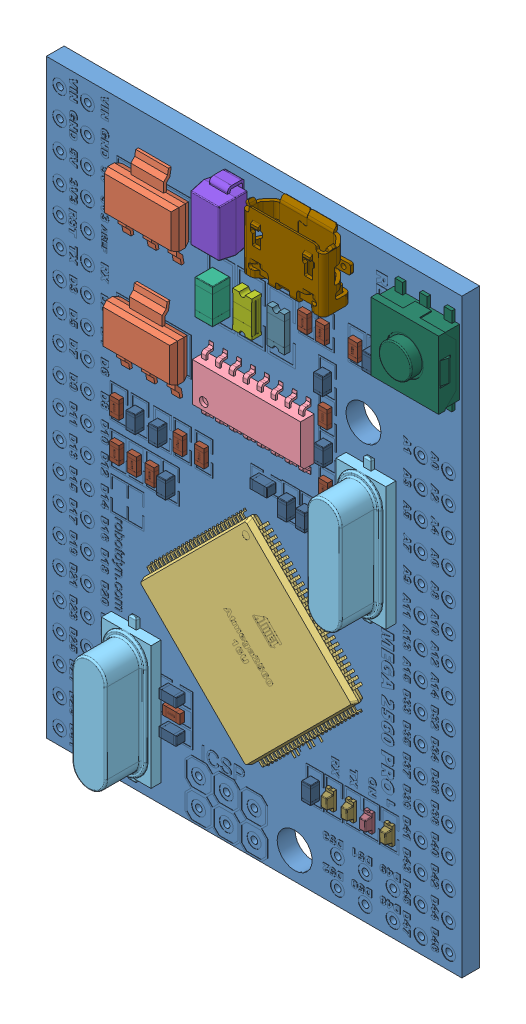
SolidWorks assembly MEGA 2560 PRO (EMBED), configuration Default. Lengths in mm.
Overall size (38 54.09 6.02).
44 component instances, 15 part files, 0 mates.
Components (placement in the parent):
- MEGA 2560 PRO (EMBED)(2)^MEGA 2560 PRO (EMBED)-1: MEGA 2560 PRO (EMBED)(2)^MEGA 2560 PRO (EMBED) [Default] at origin size (38 54.09 6.02) (virtual)
  - Mega 2560 Pro - Board^MEGA 2560 PRO (EMBED)(2)_MEGA 2560 PRO (EMBED)-1: Mega 2560 Pro - Board^MEGA 2560 PRO (EMBED)(2)_MEGA 2560 PRO (EMBED) [Default] at origin size (38 54 1.78) (virtual)
  - SOT223-3^MEGA 2560 PRO (EMBED)(2)_MEGA 2560 PRO (EMBED)-1: SOT223-3^MEGA 2560 PRO (EMBED)(2)_MEGA 2560 PRO (EMBED) [Default] at (-7.7036 13.3224 1.6256) x (-1 0 0) z (0 0 1) size (6.5 7.07 1.6) (virtual)
  - SOT223-3^MEGA 2560 PRO (EMBED)(2)_MEGA 2560 PRO (EMBED)-2: SOT223-3^MEGA 2560 PRO (EMBED)(2)_MEGA 2560 PRO (EMBED) [Default] at (-7.5781 23.9617 1.6256) x (-1 0 0) z (0 0 1) size (6.5 7.07 1.6) (virtual)
  - ATmega2560-16AU^MEGA 2560 PRO (EMBED)(2)_MEGA 2560 PRO (EMBED)-1: ATmega2560-16AU^MEGA 2560 PRO (EMBED)(2)_MEGA 2560 PRO (EMBED) [Default] at (0.2253 -9.3836 1.5256) x (0.707107 -0.707107 0) z (0 0 1) size (16 16 1.21) (virtual)
  - SOIC -16^MEGA 2560 PRO (EMBED)(2)_MEGA 2560 PRO (EMBED)-1: SOIC -16^MEGA 2560 PRO (EMBED)(2)_MEGA 2560 PRO (EMBED) [Default] at (0.546 8.9647 1.4756) x (0 1 0) z (1 0 0) size (6 1.4 9.9) (virtual)
  - Crystal Oscillator (SMD)^MEGA 2560 PRO (EMBED)(2)_MEGA 2560 PRO (EMBED)-1: Crystal Oscillator (SMD)^MEGA 2560 PRO (EMBED)(2)_MEGA 2560 PRO (EMBED) [Default] at (-10.7852 -19.6364 2.54) x (0 -1 0) z (0 0 1) size (13.06 4.55 4.32) (virtual)
  - Crystal Oscillator (SMD)^MEGA 2560 PRO (EMBED)(2)_MEGA 2560 PRO (EMBED)-2: Crystal Oscillator (SMD)^MEGA 2560 PRO (EMBED)(2)_MEGA 2560 PRO (EMBED) [Default] at (10.6809 3.6875 2.54) x (0 -1 0) z (0 0 1) size (13.06 4.55 4.32) (virtual)
  - 1206 Capacitor^MEGA 2560 PRO (EMBED)(2)_MEGA 2560 PRO (EMBED)-1: 1206 Capacitor^MEGA 2560 PRO (EMBED)(2)_MEGA 2560 PRO (EMBED) [Default] at (-3.8106 17.9279 1.6231) x (0 -1 0) z (0 0 1) size (3.2 1.6 1.6) (virtual)
  - Fuse (1206) - Green^MEGA 2560 PRO (EMBED)(2)_MEGA 2560 PRO (EMBED)-1: Fuse (1206) - Green^MEGA 2560 PRO (EMBED)(2)_MEGA 2560 PRO (EMBED) [Default] at (-0.2207 16.3875 1.6281) x (0 -1 0) z (0 0 1) size (3.28 1.75 0.87) (virtual)
  - Diode - SMD - DO-214AC^MEGA 2560 PRO (EMBED)(2)_MEGA 2560 PRO (EMBED)-1: Diode - SMD - DO-214AC^MEGA 2560 PRO (EMBED)(2)_MEGA 2560 PRO (EMBED) [Default] at (-1.7706 25.543 1.4756) x (0 -1 0) z (0 0 1) size (5.6 2.95 2.91) (virtual)
  - USB - Micro^MEGA 2560 PRO (EMBED)(2)_MEGA 2560 PRO (EMBED)-1: USB - Micro^MEGA 2560 PRO (EMBED)(2)_MEGA 2560 PRO (EMBED) [Default] at (2.2104 21.1734 1.3475) x (-1 0 0) z (0 1 0) size (7.92 3.01 5.67) (virtual)
  - 0603 Capacitor^MEGA 2560 PRO (EMBED)(2)_MEGA 2560 PRO (EMBED)-1: 0603 Capacitor^MEGA 2560 PRO (EMBED)(2)_MEGA 2560 PRO (EMBED) [Default] at (10.7145 18.9901 1.6231) x (0 -1 0) z (0 0 1) size (1.6 0.84 0.84) (virtual)
  - 0603 Capacitor^MEGA 2560 PRO (EMBED)(2)_MEGA 2560 PRO (EMBED)-2: 0603 Capacitor^MEGA 2560 PRO (EMBED)(2)_MEGA 2560 PRO (EMBED) [Default] at (4.611 3.4374 1.6231) x (0 -1 0) z (0 0 1) size (1.6 0.84 0.84) (virtual)
  - 0603 Capacitor^MEGA 2560 PRO (EMBED)(2)_MEGA 2560 PRO (EMBED)-3: 0603 Capacitor^MEGA 2560 PRO (EMBED)(2)_MEGA 2560 PRO (EMBED) [Default] at (7.1573 7.8647 1.6231) x (0 1 0) z (0 0 1) size (1.6 0.84 0.84) (virtual)
  - 0603 Capacitor^MEGA 2560 PRO (EMBED)(2)_MEGA 2560 PRO (EMBED)-4: 0603 Capacitor^MEGA 2560 PRO (EMBED)(2)_MEGA 2560 PRO (EMBED) [Default] at (7.0977 13.4599 1.6231) x (0 1 0) z (0 0 1) size (1.6 0.84 0.84) (virtual)
  - 0603 Capacitor^MEGA 2560 PRO (EMBED)(2)_MEGA 2560 PRO (EMBED)-5: 0603 Capacitor^MEGA 2560 PRO (EMBED)(2)_MEGA 2560 PRO (EMBED) [Default] at (5.1576 -19.4722 1.6231) x (0 1 0) z (1 0 0) size (1.6 0.84 0.84) (virtual)
  - 0603 Capacitor^MEGA 2560 PRO (EMBED)(2)_MEGA 2560 PRO (EMBED)-6: 0603 Capacitor^MEGA 2560 PRO (EMBED)(2)_MEGA 2560 PRO (EMBED) [Default] at (-10.8858 1.8771 1.6231) x (0 1 0) z (1 0 0) size (1.6 0.84 0.84) (virtual)
  - 0603 Capacitor^MEGA 2560 PRO (EMBED)(2)_MEGA 2560 PRO (EMBED)-7: 0603 Capacitor^MEGA 2560 PRO (EMBED)(2)_MEGA 2560 PRO (EMBED) [Default] at (2.9599 3.4697 1.6231) x (0 -1 0) z (0 0 1) size (1.6 0.84 0.84) (virtual)
  - 0603 Capacitor^MEGA 2560 PRO (EMBED)(2)_MEGA 2560 PRO (EMBED)-8: 0603 Capacitor^MEGA 2560 PRO (EMBED)(2)_MEGA 2560 PRO (EMBED) [Default] at (2.0157 3.7447 1.6231) x (-1 0 0) z (0 0 1) size (1.6 0.84 0.84) (virtual)
  - 0603 Capacitor^MEGA 2560 PRO (EMBED)(2)_MEGA 2560 PRO (EMBED)-9: 0603 Capacitor^MEGA 2560 PRO (EMBED)(2)_MEGA 2560 PRO (EMBED) [Default] at (-8.0885 -1.9063 1.6231) x (0 1 0) z (1 0 0) size (1.6 0.84 0.84) (virtual)
  - 0603 Capacitor^MEGA 2560 PRO (EMBED)(2)_MEGA 2560 PRO (EMBED)-10: 0603 Capacitor^MEGA 2560 PRO (EMBED)(2)_MEGA 2560 PRO (EMBED) [Default] at (-3.7884 20.5934 1.6231) x (0 1 0) z (0 0 1) size (1.6 0.84 0.84) (virtual)
  - 0603 Capacitor^MEGA 2560 PRO (EMBED)(2)_MEGA 2560 PRO (EMBED)-11: 0603 Capacitor^MEGA 2560 PRO (EMBED)(2)_MEGA 2560 PRO (EMBED) [Default] at (-8.8216 3.4762 1.6231) x (0 -1 0) z (0 0 1) size (1.6 0.84 0.84) (virtual)
  - 0603 Capacitor^MEGA 2560 PRO (EMBED)(2)_MEGA 2560 PRO (EMBED)-12: 0603 Capacitor^MEGA 2560 PRO (EMBED)(2)_MEGA 2560 PRO (EMBED) [Default] at (6.3032 3.4697 2.4613) x (0 -1 0) z (1 0 0) size (1.6 0.84 0.84) (virtual)
  - 0603 Capacitor^MEGA 2560 PRO (EMBED)(2)_MEGA 2560 PRO (EMBED)-13: 0603 Capacitor^MEGA 2560 PRO (EMBED)(2)_MEGA 2560 PRO (EMBED) [Default] at (-6.2819 -20.9115 1.6231) x (-1 0 0) z (0 1 0) size (1.6 0.84 0.84) (virtual)
  - 0603 Capacitor^MEGA 2560 PRO (EMBED)(2)_MEGA 2560 PRO (EMBED)-14: 0603 Capacitor^MEGA 2560 PRO (EMBED)(2)_MEGA 2560 PRO (EMBED) [Default] at (-7.8888 -17.889 1.6231) size (1.6 0.84 0.84) (virtual)
  - 0603 Resistor^MEGA 2560 PRO (EMBED)(2)_MEGA 2560 PRO (EMBED)-1: 0603 Resistor^MEGA 2560 PRO (EMBED)(2)_MEGA 2560 PRO (EMBED) [Default] at (-6.1185 1.9325 1.6231) x (0 1 0) z (0 0 1) size (1.6 0.85 0.56) (virtual)
  - 0603 Resistor^MEGA 2560 PRO (EMBED)(2)_MEGA 2560 PRO (EMBED)-2: 0603 Resistor^MEGA 2560 PRO (EMBED)(2)_MEGA 2560 PRO (EMBED) [Default] at (-8.697 -1.8307 1.6231) x (0 1 0) z (0 0 1) size (1.6 0.85 0.56) (virtual)
  - 0603 Resistor^MEGA 2560 PRO (EMBED)(2)_MEGA 2560 PRO (EMBED)-3: 0603 Resistor^MEGA 2560 PRO (EMBED)(2)_MEGA 2560 PRO (EMBED) [Default] at (-10.3133 -1.7908 1.6231) x (0 1 0) z (0 0 1) size (1.6 0.85 0.56) (virtual)
  - 0603 Resistor^MEGA 2560 PRO (EMBED)(2)_MEGA 2560 PRO (EMBED)-4: 0603 Resistor^MEGA 2560 PRO (EMBED)(2)_MEGA 2560 PRO (EMBED) [Default] at (6.8981 17.2332 1.6231) x (0 1 0) z (0 0 1) size (1.6 0.85 0.56) (virtual)
  - 0603 Resistor^MEGA 2560 PRO (EMBED)(2)_MEGA 2560 PRO (EMBED)-5: 0603 Resistor^MEGA 2560 PRO (EMBED)(2)_MEGA 2560 PRO (EMBED) [Default] at (-4.1536 1.9449 1.6231) x (0 1 0) z (0 0 1) size (1.6 0.85 0.56) (virtual)
  - 0603 Resistor^MEGA 2560 PRO (EMBED)(2)_MEGA 2560 PRO (EMBED)-6: 0603 Resistor^MEGA 2560 PRO (EMBED)(2)_MEGA 2560 PRO (EMBED) [Default] at (7.1292 10.6782 1.6231) x (0 1 0) z (0 0 1) size (1.6 0.85 0.56) (virtual)
  - 0603 Resistor^MEGA 2560 PRO (EMBED)(2)_MEGA 2560 PRO (EMBED)-7: 0603 Resistor^MEGA 2560 PRO (EMBED)(2)_MEGA 2560 PRO (EMBED) [Default] at (5.2754 17.2903 1.6231) x (0 1 0) z (0 0 1) size (1.6 0.85 0.56) (virtual)
  - 0603 Resistor^MEGA 2560 PRO (EMBED)(2)_MEGA 2560 PRO (EMBED)-8: 0603 Resistor^MEGA 2560 PRO (EMBED)(2)_MEGA 2560 PRO (EMBED) [Default] at (9.8818 17.3443 1.6231) x (0 1 0) z (0 0 1) size (1.6 0.85 0.56) (virtual)
  - 0603 Resistor^MEGA 2560 PRO (EMBED)(2)_MEGA 2560 PRO (EMBED)-9: 0603 Resistor^MEGA 2560 PRO (EMBED)(2)_MEGA 2560 PRO (EMBED) [Default] at (-11.9263 1.9088 1.6231) x (0 1 0) z (0 0 1) size (1.6 0.85 0.56) (virtual)
  - 0603 Resistor^MEGA 2560 PRO (EMBED)(2)_MEGA 2560 PRO (EMBED)-10: 0603 Resistor^MEGA 2560 PRO (EMBED)(2)_MEGA 2560 PRO (EMBED) [Default] at (7.18 4.9009 1.6231) x (0 1 0) z (0 0 1) size (1.6 0.85 0.56) (virtual)
  - 0603 Resistor^MEGA 2560 PRO (EMBED)(2)_MEGA 2560 PRO (EMBED)-11: 0603 Resistor^MEGA 2560 PRO (EMBED)(2)_MEGA 2560 PRO (EMBED) [Default] at (-11.9146 -1.6797 1.6231) x (0 1 0) z (0 0 1) size (1.6 0.85 0.56) (virtual)
  - 0603 Resistor^MEGA 2560 PRO (EMBED)(2)_MEGA 2560 PRO (EMBED)-12: 0603 Resistor^MEGA 2560 PRO (EMBED)(2)_MEGA 2560 PRO (EMBED) [Default] at (-6.3495 -18.5603 1.6231) x (-1 0 0) z (0 0 1) size (1.6 0.85 0.56) (virtual)
  - LED - 0603 - Blue^MEGA 2560 PRO (EMBED)(2)_MEGA 2560 PRO (EMBED)-1: LED - 0603 - Blue^MEGA 2560 PRO (EMBED)(2)_MEGA 2560 PRO (EMBED) [Default] at (7.1908 -19.2239 1.6256) x (0 1 0) z (0 0 1) size (1.63 0.73 0.83) (virtual)
  - LED_-_Vishay_-_6063_-_Green^MEGA 2560 PRO (EMBED)(2)_MEGA 2560 PRO (EMBED)-1: LED_-_Vishay_-_6063_-_Green^MEGA 2560 PRO (EMBED)(2)_MEGA 2560 PRO (EMBED) [Default] at (10.6783 -18.0475 1.5956) x (0 -1 0) z (0 0 1) size (1.63 0.73 0.83) (virtual)
  - LED - 0603 - Blue^MEGA 2560 PRO (EMBED)(2)_MEGA 2560 PRO (EMBED)-2: LED - 0603 - Blue^MEGA 2560 PRO (EMBED)(2)_MEGA 2560 PRO (EMBED) [Default] at (9.0246 -17.9783 1.6256) x (0 -1 0) z (0 0 1) size (1.63 0.73 0.83) (virtual)
  - 1206 Fuse^MEGA 2560 PRO (EMBED)(2)_MEGA 2560 PRO (EMBED)-1: 1206 Fuse^MEGA 2560 PRO (EMBED)(2)_MEGA 2560 PRO (EMBED) [Default] at (1.6964 17.9461 1.6231) x (0 -1 0) z (0 0 1) size (3.2 1.6 0.53) (virtual)
  - SWT-32^MEGA 2560 PRO (EMBED)(2)_MEGA 2560 PRO (EMBED)-1: SWT-32^MEGA 2560 PRO (EMBED)(2)_MEGA 2560 PRO (EMBED) [Default] at (15.7781 21.6695 1.6256) x (0 1 0) z (0 0 1) size (8 6.4 2.9) (virtual)
  - LED - 0603 - Blue^MEGA 2560 PRO (EMBED)(2)_MEGA 2560 PRO (EMBED)-3: LED - 0603 - Blue^MEGA 2560 PRO (EMBED)(2)_MEGA 2560 PRO (EMBED) [Default] at (12.5463 -18.1103 1.6256) x (0 -1 0) z (0 0 1) size (1.63 0.73 0.83) (virtual)
